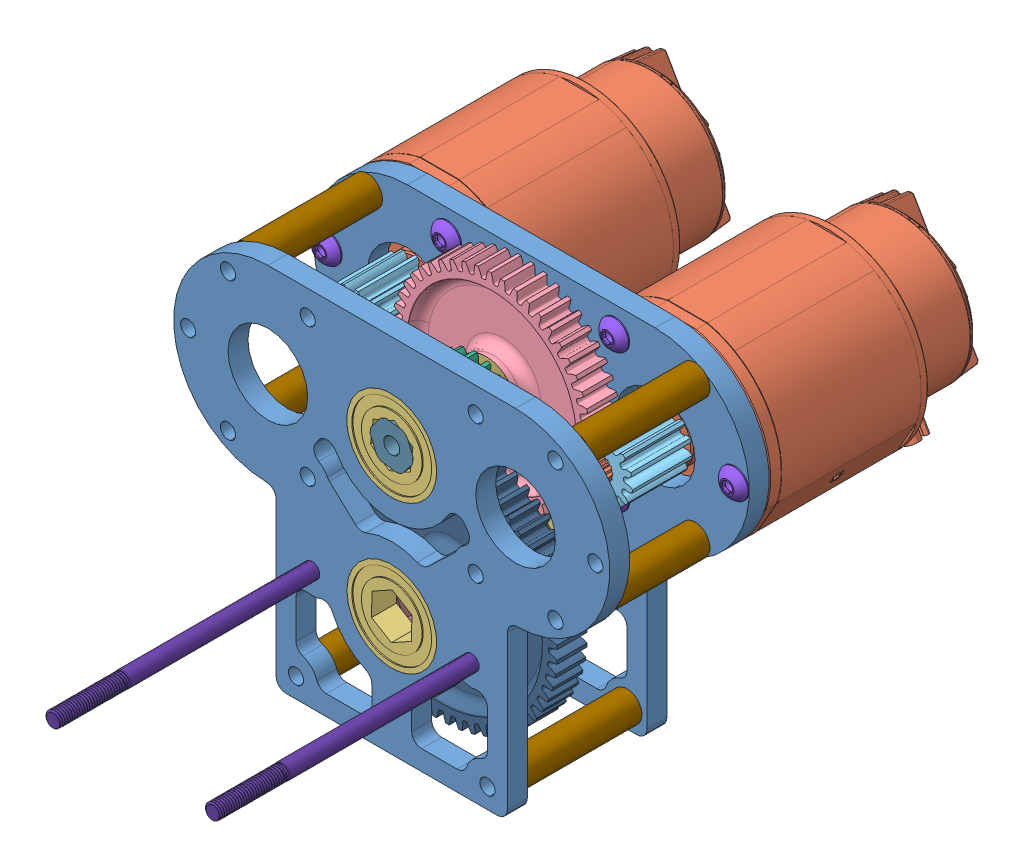
SolidWorks assembly 2 stage elevator gearbox, configuration Default. Lengths in mm.
Overall size (160.87 135.08 215.73).
38 component instances, 17 part files, 79 mates.
Components (placement in the parent):
- 2stage gearbox plate-1: 2stage gearbox plate [Default] at (38.8703 49.9501 110.3319) size (138.89 115.16 6.35)
- Vexpro - Falcon 500 - 217-6515-1: Vexpro - Falcon 500 - 217-6515 [Default] at (74.1311 92.2322 73.3938) x (0.866025 -0.5 0) z (0 0 1) size (60.01 60.01 116.76)
- Vexpro - Falcon 500 - 217-6515-2: Vexpro - Falcon 500 - 217-6515 [Default] at (-4.7613 92.2322 73.3938) x (0.866025 -0.5 0) z (0 0 1) size (60.01 60.01 116.76)
- Vexpro - .5in hex bearing flanged - 217-3875-1: Vexpro - .5in hex bearing flanged - 217-3875 [Default] at (38.8703 97.0163 110.3319) x (0.982389 0.186848 0) z (0.186848 -0.982389 0) size (31.12 7.94 31.12)
- Vexpro - .5in hex bearing flanged - 217-3875-2: Vexpro - .5in hex bearing flanged - 217-3875 [Default] at (38.8703 49.9501 110.3319) x (0.9326 0.360911 0) z (0.360911 -0.9326 0) size (31.12 7.94 31.12)
- 48t pocketed gear-1: 48t pocketed gear [Default] at (38.8703 97.0163 124.594) x (0.984542 -0.175146 0) z (0 0 1) size (63.43 63.43 12.65)
- 14t pinion-1: 14t pinion [Default] at (78.3161 97.0172 124.4944) x (0.865876 0.500258 0) z (0 0 1) size (20.01 20.32 19.05)
- 14t pinion-2: 14t pinion [Default] at (-0.5766 97.0171 124.4944) x (0.709301 0.704906 0) z (0 0 1) size (20.01 20.32 19.05)
- Vexpro - 18t 20DP .5 Hex Gear - 217-5460-1: Vexpro - 18t 20DP .5 Hex Gear - 217-5460 [Default] at (38.8703 97.0163 140.5444) x (0.941397 0.3373 0) z (0 0 1) size (25.18 25.4 12.6)
- Vexpro - .5in acetal hex spacer - 217 - 3261-1: Vexpro - .5in acetal hex spacer - 217 - 3261 [Default] at (38.8703 49.9501 124.6194) x (-0.39458 0.918862 0) z (0 0 1) size (19.5 19.5 12.7)
- 2stage gearbox plate-2: 2stage gearbox plate [outside] at (38.8703 49.9501 154.7819) size (138.89 115.16 6.35)
- Vexpro - .5in hex bearing flanged - 217-3875-4: Vexpro - .5in hex bearing flanged - 217-3875 [Default] at (38.8703 49.9501 161.1319) x (-0.017353 -0.999849 0) z (0.999849 -0.017353 0) size (31.12 7.94 31.12)
- Vexpro - .5in hex bearing flanged - 217-3875-5: Vexpro - .5in hex bearing flanged - 217-3875 [Default] at (38.8703 97.0163 161.1319) x (-0.113044 -0.99359 0) z (0.99359 -0.113044 0) size (31.12 7.94 31.12)
- McMaster - 10-32 .3125in button head screw - 97763A706-2: McMaster - 10-32 .3125in button head screw - 97763A706 [97763A706] at (12.1241 119.0134 113.9959) size (9.17 9.17 10.95)
- McMaster - 10-32 .3125in button head screw - 97763A706-3: McMaster - 10-32 .3125in button head screw - 97763A706 [97763A706] at (12.1241 75.0193 113.9959) size (9.17 9.17 10.95)
- McMaster - 10-32 .3125in button head screw - 97763A706-4: McMaster - 10-32 .3125in button head screw - 97763A706 [97763A706] at (-25.9759 97.0163 113.9959) size (9.17 9.17 10.95)
- McMaster - 10-32 .3125in button head screw - 97763A706-5: McMaster - 10-32 .3125in button head screw - 97763A706 [97763A706] at (-13.2759 75.0193 113.9959) size (9.17 9.17 10.95)
- McMaster - 10-32 .3125in button head screw - 97763A706-9: McMaster - 10-32 .3125in button head screw - 97763A706 [97763A706] at (103.7165 97.0163 113.9959) size (9.17 9.17 10.95)
- McMaster - 10-32 .3125in button head screw - 97763A706-10: McMaster - 10-32 .3125in button head screw - 97763A706 [97763A706] at (65.6165 75.0193 113.9959) size (9.17 9.17 10.95)
- McMaster - 10-32 .3125in button head screw - 97763A706-12: McMaster - 10-32 .3125in button head screw - 97763A706 [97763A706] at (65.6165 119.0134 113.9959) size (9.17 9.17 10.95)
- McMaster - 10-32 .3125in button head screw - 97763A706-13: McMaster - 10-32 .3125in button head screw - 97763A706 [97763A706] at (8.3903 18.2001 113.018) x (-0.932553 0.361034 0) z (0 0 -1) size (9.17 9.17 10.95)
- McMaster - 10-32 .3125in button head screw - 97763A706-15: McMaster - 10-32 .3125in button head screw - 97763A706 [97763A706] at (69.3503 18.2001 113.018) x (-0.932553 0.361034 0) z (0 0 -1) size (9.17 9.17 10.95)
- 1.5in gearbox spacer-1: 1.5in gearbox spacer [Default] at (69.3503 18.2001 154.7819) x (-0.965755 0.259455 0) z (-0.259455 -0.965755 0) size (9.53 38.1 9.53)
- 1.5in gearbox spacer-2: 1.5in gearbox spacer [Default] at (8.3903 18.2001 154.7819) x (-0.965755 0.259455 0) z (-0.259455 -0.965755 0) size (9.53 38.1 9.53)
- 1.5in gearbox spacer-3: 1.5in gearbox spacer [Default] at (91.0165 119.0134 154.7819) x (-0.883824 -0.46782 0) z (0.46782 -0.883824 0) size (9.53 38.1 9.53)
- 1.5in gearbox spacer-4: 1.5in gearbox spacer [Default] at (-13.2759 119.0134 154.7819) x (-0.965755 0.259455 0) z (-0.259455 -0.965755 0) size (9.53 38.1 9.53)
- 1.5in gearbox spacer-5: 1.5in gearbox spacer [Default] at (-13.2759 75.0193 154.7819) x (-0.965755 0.259455 0) z (-0.259455 -0.965755 0) size (9.53 38.1 9.53)
- 56t pocketed gear-1: 56t pocketed gear [Default] at (38.8703 49.9501 140.4444) x (0.941864 -0.335993 0) z (0 0 1) size (73.6 73.6 12.6)
- Clamping Shaft Collar - 1_2 Hex ID (217-2737)-1: Clamping Shaft Collar - 1_2 Hex ID (217-2737) [Default] at (38.8703 97.0163 150.0194) x (0.340948 -0.940082 0) z (0 0 1) size (25.39 25.4 6.35)
- Vexpro - .125 acetal hex spacer - 217-2758-1: Vexpro - .125 acetal hex spacer - 217-2758 [Default] at (38.8703 49.9501 132.5569) x (0.658563 0.752525 0) z (0 0 1) size (19.05 19.05 3.17)
- Vexpro - .125 acetal hex spacer - 217-2758-2: Vexpro - .125 acetal hex spacer - 217-2758 [Default] at (38.8703 97.0163 132.6569) x (0.658563 0.752525 0) z (0 0 1) size (19.05 19.05 3.17)
- Vexpro - .25in acetal hex spacer - 217-3259-1: Vexpro - .25in acetal hex spacer - 217-3259 [Default] at (38.8703 49.9501 150.0194) size (19.5 19.5 6.35)
- 2in hex axle-1: 2in hex axle [Default] at (64.1668 94.7262 213.5194) x (0.995927 -0.090161 0) z (0 0 1) size (14.65 14.61 50.8)
- McMaster - .25 ID washer - 96765A140-1: McMaster - .25 ID washer - 96765A140 [96765A140] at (38.8703 97.0163 110.3319) x (1 0 0) z (0 1 0) size (15.88 1.52 15.88)
- McMaster - .25-20 .5in socket head - 91251A537-1: McMaster - .25-20 .5in socket head - 91251A537 [91251A537] at (38.8703 97.0163 121.5079) size (9.53 9.53 20.44)
- McMaster 10-32 3.tin socket Head 91251A361_Black-Oxide Alloy Steel Socket Head Screw-2: McMaster 10-32 3.tin socket Head 91251A361_Black-Oxide Alloy Steel Socket Head Screw [91251A361] at (13.4703 49.9501 196.8189) x (0.923728 0.383049 0) z (0 0 -1) size (7.94 7.94 94.22)
- McMaster 10-32 3.tin socket Head 91251A361_Black-Oxide Alloy Steel Socket Head Screw-3: McMaster 10-32 3.tin socket Head 91251A361_Black-Oxide Alloy Steel Socket Head Screw [91251A361] at (64.2703 49.9501 196.8189) x (0.923728 0.383049 0) z (0 0 -1) size (7.94 7.94 94.22)
- 1.5in gearbox spacer-6: 1.5in gearbox spacer [Default] at (91.0165 75.0193 154.7819) x (-0.883824 -0.46782 0) z (0.46782 -0.883824 0) size (9.53 38.1 9.53)
Mates (geometry in assembly coordinates):
- Concentric1: concentric aligned: cylinder of Vexpro - Falcon 500 - 217-6515-1 through (78.3165 97.0163 106.3319) axis (0 0 -1) radius 30; cylinder of 2stage gearbox plate-1 through (78.3165 97.0163 116.6819) axis (0 0 -1) radius 29.9974
- Concentric2: concentric aligned: cylinder of Vexpro - Falcon 500 - 217-6515-2 through (-0.5759 97.0163 106.3319) axis (0 0 -1) radius 30; cylinder of 2stage gearbox plate-1 through (-0.5759 97.0163 116.6819) axis (0 0 -1) radius 29.9974
- Coincident1: coincident anti-aligned: plane of 2stage gearbox plate-1 through (38.8703 49.9501 110.3319) normal (0 0 -1); plane of Vexpro - Falcon 500 - 217-6515-2 through (-8.8248 92.2538 110.3319) normal (0 0 1)
- Coincident2: coincident anti-aligned: plane of 2stage gearbox plate-1 through (38.8703 49.9501 110.3319) normal (0 0 -1); plane of Vexpro - Falcon 500 - 217-6515-1 through (70.0676 92.2538 110.3319) normal (0 0 1)
- Coincident3: coincident anti-aligned: plane of 2stage gearbox plate-1 through (38.8703 49.9501 116.6819) normal (0 0 1); plane of Vexpro - .5in hex bearing flanged - 217-3875-1 through (54.1538 99.9232 116.6819) normal (0 0 -1)
- Coincident4: coincident anti-aligned: plane of 2stage gearbox plate-1 through (38.8703 49.9501 116.6819) normal (0 0 1); plane of Vexpro - .5in hex bearing flanged - 217-3875-2 through (53.3792 55.565 116.6819) normal (0 0 -1)
- Concentric6: concentric anti-aligned: circle of Vexpro - .5in hex bearing flanged - 217-3875-1; unknown of 48t pocketed gear-1
- Concentric7: concentric: point of Vexpro - Falcon 500 - 217-6515-1; unknown of 14t pinion-1
- Coincident6: coincident anti-aligned: plane of Vexpro - Falcon 500 - 217-6515-1 through (80.4098 94.8914 114.9694) normal (0 0 1); plane of 14t pinion-1 through (73.2334 105.8145 114.9694) normal (0 0 -1)
- Concentric8: concentric: cylinder of Vexpro - Falcon 500 - 217-6515-2 through (-0.5759 97.0163 145.1319) axis (0 0 1) radius 1.7272; unknown of 14t pinion-2
- Coincident8: coincident anti-aligned: plane of Vexpro - Falcon 500 - 217-6515-2 through (1.5174 94.8914 114.9694) normal (0 0 1); plane of 14t pinion-2 through (-7.7384 104.2236 114.9694) normal (0 0 -1)
- Concentric11: concentric aligned: unknown of 48t pocketed gear-1; unknown of Vexpro - 18t 20DP .5 Hex Gear - 217-5460-1
- Concentric12: concentric anti-aligned: unknown of Vexpro - .5in hex bearing flanged - 217-3875-2; cylinder of Vexpro - .5in acetal hex spacer - 217 - 3261-1 through (38.8703 49.9501 130.9694) axis (0 0 -1) radius 9.75
- Concentric13: concentric aligned: unknown of Vexpro - 18t 20DP .5 Hex Gear - 217-5460-1; cylinder of 2stage gearbox plate-2 through (38.8703 97.0163 161.1319) axis (0 0 -1) radius 14.2875
- Concentric14: concentric anti-aligned: cylinder of Vexpro - Falcon 500 - 217-6515-2 through (-0.5759 97.0163 145.1319) axis (0 0 1) radius 1.7272; cylinder of 2stage gearbox plate-2 through (-0.5759 97.0163 161.1319) axis (0 0 -1) radius 12.7
- Concentric15: concentric aligned: cylinder of 2stage gearbox plate-2 through (38.8703 49.9501 161.1319) axis (0 0 -1) radius 14.2875; cylinder of Vexpro - .5in hex bearing flanged - 217-3875-4 through (38.8703 49.9501 161.1319) axis (0 0 -1) radius 14.2748
- Coincident12: coincident anti-aligned: plane of 2stage gearbox plate-2 through (38.8703 49.9501 154.7819) normal (0 0 -1); plane of Vexpro - .5in hex bearing flanged - 217-3875-4 through (38.6003 34.395 154.7819) normal (0 0 1)
- Concentric16: concentric aligned: cylinder of Vexpro - .5in hex bearing flanged - 217-3875-5 through (38.8703 97.0163 161.1319) axis (0 0 -1) radius 14.2748; cylinder of 2stage gearbox plate-2 through (38.8703 97.0163 161.1319) axis (0 0 -1) radius 14.2875
- Coincident13: coincident anti-aligned: plane of 2stage gearbox plate-2 through (38.8703 49.9501 154.7819) normal (0 0 -1); plane of Vexpro - .5in hex bearing flanged - 217-3875-5 through (37.1116 81.5585 154.7819) normal (0 0 1)
- Concentric17: concentric aligned: unknown of Vexpro - Falcon 500 - 217-6515-2; unknown of McMaster - 10-32 .3125in button head screw - 97763A706-4
- Concentric18: concentric aligned: unknown of Vexpro - Falcon 500 - 217-6515-1; unknown of McMaster - 10-32 .3125in button head screw - 97763A706-12
- Concentric21: concentric aligned: cylinder of 2stage gearbox plate-1 through (12.1241 119.0134 110.3319) axis (0 0 1) radius 2.413; unknown of McMaster - 10-32 .3125in button head screw - 97763A706-2
- Coincident18: coincident anti-aligned: plane of 2stage gearbox plate-1 through (38.8703 49.9501 116.6819) normal (0 0 1); plane of McMaster - 10-32 .3125in button head screw - 97763A706-2 through (12.1241 123.5981 116.6819) normal (0 0 -1)
- Coincident19: coincident anti-aligned: plane of 2stage gearbox plate-1 through (38.8703 49.9501 116.6819) normal (0 0 1); plane of McMaster - 10-32 .3125in button head screw - 97763A706-3 through (12.1241 79.604 116.6819) normal (0 0 -1)
- Concentric22: concentric aligned: cylinder of 2stage gearbox plate-1 through (12.1241 75.0193 110.3319) axis (0 0 1) radius 2.413; unknown of McMaster - 10-32 .3125in button head screw - 97763A706-3
- Concentric23: concentric aligned: cylinder of 2stage gearbox plate-1 through (-25.9759 97.0163 110.3319) axis (0 0 1) radius 2.413; unknown of McMaster - 10-32 .3125in button head screw - 97763A706-4
- Coincident20: coincident anti-aligned: plane of 2stage gearbox plate-1 through (38.8703 49.9501 116.6819) normal (0 0 1); plane of McMaster - 10-32 .3125in button head screw - 97763A706-4 through (-25.9759 101.601 116.6819) normal (0 0 -1)
- Concentric24: concentric aligned: cylinder of 2stage gearbox plate-1 through (-13.2759 75.0193 110.3319) axis (0 0 1) radius 2.413; unknown of McMaster - 10-32 .3125in button head screw - 97763A706-5
- Coincident21: coincident anti-aligned: plane of 2stage gearbox plate-1 through (38.8703 49.9501 116.6819) normal (0 0 1); plane of McMaster - 10-32 .3125in button head screw - 97763A706-5 through (-13.2759 79.604 116.6819) normal (0 0 -1)
- Coincident23: coincident anti-aligned: plane of 2stage gearbox plate-1 through (38.8703 49.9501 116.6819) normal (0 0 1); plane of McMaster - 10-32 .3125in button head screw - 97763A706-12 through (65.6165 123.5981 116.6819) normal (0 0 -1)
- Concentric27: concentric aligned: cylinder of 2stage gearbox plate-1 through (65.6165 119.0134 110.3319) axis (0 0 1) radius 2.413; unknown of McMaster - 10-32 .3125in button head screw - 97763A706-12
- Coincident25: coincident anti-aligned: plane of 2stage gearbox plate-1 through (38.8703 49.9501 116.6819) normal (0 0 1); plane of McMaster - 10-32 .3125in button head screw - 97763A706-9 through (103.7165 101.601 116.6819) normal (0 0 -1)
- Concentric29: concentric aligned: cylinder of 2stage gearbox plate-1 through (103.7165 97.0163 110.3319) axis (0 0 1) radius 2.413; unknown of McMaster - 10-32 .3125in button head screw - 97763A706-9
- Concentric30: concentric aligned: unknown of McMaster - 10-32 .3125in button head screw - 97763A706-10; cylinder of 2stage gearbox plate-1 through (65.6165 75.0193 110.3319) axis (0 0 1) radius 2.413
- Coincident26: coincident anti-aligned: plane of 2stage gearbox plate-1 through (38.8703 49.9501 116.6819) normal (0 0 1); plane of McMaster - 10-32 .3125in button head screw - 97763A706-10 through (65.6165 79.604 116.6819) normal (0 0 -1)
- Coincident28: coincident anti-aligned: plane of 2stage gearbox plate-1 through (38.8703 49.9501 110.3319) normal (0 0 -1); plane of McMaster - 10-32 .3125in button head screw - 97763A706-13 through (10.0455 22.4756 110.3319) normal (0 0 1)
- Concentric32: concentric aligned: unknown of McMaster - 10-32 .3125in button head screw - 97763A706-13; unknown of 2stage gearbox plate-1
- Coincident29: coincident anti-aligned: plane of 2stage gearbox plate-1 through (38.8703 49.9501 110.3319) normal (0 0 -1); plane of McMaster - 10-32 .3125in button head screw - 97763A706-15 through (71.0055 22.4756 110.3319) normal (0 0 1)
- Concentric33: concentric aligned: unknown of McMaster - 10-32 .3125in button head screw - 97763A706-15; cylinder of 2stage gearbox plate-1 through (69.3503 18.2001 116.6819) axis (0 0 -1) radius 2.413
- Concentric40: concentric anti-aligned: cylinder of 1.5in gearbox spacer-1 through (69.3503 18.2001 116.6819) axis (0 0 1) radius 4.7625; cylinder of 2stage gearbox plate-2 through (69.3503 18.2001 161.1319) axis (0 0 -1) radius 2.413
- Coincident37: coincident anti-aligned: plane of 2stage gearbox plate-2 through (38.8703 49.9501 154.7819) normal (0 0 -1); plane of 1.5in gearbox spacer-1 through (69.3503 18.2001 154.7819) normal (0 0 1)
- Coincident38: coincident anti-aligned: plane of 2stage gearbox plate-1 through (38.8703 49.9501 116.6819) normal (0 0 1); plane of 1.5in gearbox spacer-1 through (69.3503 18.2001 116.6819) normal (0 0 -1)
- Concentric41: concentric anti-aligned: cylinder of 1.5in gearbox spacer-2 through (8.3903 18.2001 116.6819) axis (0 0 1) radius 4.7625; unknown of 2stage gearbox plate-2
- Coincident39: coincident anti-aligned: plane of 2stage gearbox plate-2 through (38.8703 49.9501 154.7819) normal (0 0 -1); plane of 1.5in gearbox spacer-2 through (8.3903 18.2001 154.7819) normal (0 0 1)
- Concentric42: concentric aligned: cylinder of 1.5in gearbox spacer-3 through (91.0165 119.0134 116.6819) axis (0 0 1) radius 4.7625; unknown of 2stage gearbox plate-1
- Coincident40: coincident anti-aligned: plane of 2stage gearbox plate-2 through (38.8703 49.9501 154.7819) normal (0 0 -1); plane of 1.5in gearbox spacer-3 through (91.0165 119.0134 154.7819) normal (0 0 1)
- Concentric43: concentric aligned: cylinder of 1.5in gearbox spacer-4 through (-13.2759 119.0134 116.6819) axis (0 0 1) radius 4.7625; cylinder of 2stage gearbox plate-1 through (-13.2759 119.0134 110.3319) axis (0 0 1) radius 2.413
- Coincident41: coincident anti-aligned: plane of 2stage gearbox plate-1 through (38.8703 49.9501 116.6819) normal (0 0 1); plane of 1.5in gearbox spacer-4 through (-13.2759 119.0134 116.6819) normal (0 0 -1)
- Coincident42: coincident anti-aligned: plane of 2stage gearbox plate-2 through (38.8703 49.9501 154.7819) normal (0 0 -1); plane of 1.5in gearbox spacer-5 through (-13.2759 75.0193 154.7819) normal (0 0 1)
- Concentric45: concentric aligned: cylinder of 1.5in gearbox spacer-5 through (-13.2759 75.0193 116.6819) axis (0 0 1) radius 4.7625; unknown of 2stage gearbox plate-2
- Coincident46: coincident anti-aligned: plane of Vexpro - .5in hex bearing flanged - 217-3875-2 through (44.7923 52.2419 118.2694) normal (0 0 1); plane of Vexpro - .5in acetal hex spacer - 217 - 3261-1 through (38.8703 49.9501 118.2694) normal (0 0 -1)
- Concentric48: concentric anti-aligned: unknown of Vexpro - .5in acetal hex spacer - 217 - 3261-1; unknown of 56t pocketed gear-1
- Concentric50: concentric aligned: cylinder of Vexpro - .5in hex bearing flanged - 217-3875-5 through (38.8703 97.0163 161.1319) axis (0 0 -1) radius 15.5575; cylinder of Clamping Shaft Collar - 1_2 Hex ID (217-2737)-1 through (38.8703 97.0163 153.1944) axis (0 0 -1) radius 12.7
- Coincident54: coincident anti-aligned: plane of Vexpro - .5in hex bearing flanged - 217-3875-5 through (38.1525 90.707 153.1944) normal (0 0 -1); plane of Clamping Shaft Collar - 1_2 Hex ID (217-2737)-1 through (38.8703 97.0163 153.1944) normal (0 0 1)
- Coincident56: coincident anti-aligned: plane of Vexpro - 18t 20DP .5 Hex Gear - 217-5460-1 through (38.8703 97.0163 146.8444) normal (0 0 1); plane of Clamping Shaft Collar - 1_2 Hex ID (217-2737)-1 through (38.8703 97.0163 146.8444) normal (0 0 -1)
- Coincident58: coincident aligned: plane of Vexpro - .5in hex bearing flanged - 217-3875-1 through (45.1085 98.2028 118.2694) normal (0 0 1); circle of 48t pocketed gear-1
- Concentric52: concentric aligned: cylinder of Vexpro - .5in acetal hex spacer - 217 - 3261-1 through (38.8703 49.9501 130.9694) axis (0 0 -1) radius 9.75; cylinder of Vexpro - .125 acetal hex spacer - 217-2758-1 through (38.8703 49.9501 134.1444) axis (0 0 -1) radius 9.525
- Coincident59: coincident aligned: circle of 56t pocketed gear-1; plane of Vexpro - .125 acetal hex spacer - 217-2758-1 through (38.8703 49.9501 134.1444) normal (0 0 1)
- Coincident60: coincident aligned: plane of Vexpro - .5in acetal hex spacer - 217 - 3261-1 through (38.8703 49.9501 130.9694) normal (0 0 1); circle of Vexpro - .125 acetal hex spacer - 217-2758-1
- Concentric53: concentric aligned: cylinder of 48t pocketed gear-1 through (38.8703 97.0163 130.9186) axis (0 0 -1) radius 8.89; cylinder of Vexpro - .125 acetal hex spacer - 217-2758-2 through (38.8703 97.0163 134.2444) axis (0 0 -1) radius 9.525
- Coincident61: coincident anti-aligned: circle of Vexpro - 18t 20DP .5 Hex Gear - 217-5460-1; plane of Vexpro - .125 acetal hex spacer - 217-2758-2 through (38.8703 97.0163 134.2444) normal (0 0 1)
- Concentric54: concentric aligned: cylinder of 56t pocketed gear-1 through (38.8703 49.9501 146.7444) axis (0 0 -1) radius 8.89; cylinder of Vexpro - .25in acetal hex spacer - 217-3259-1 through (38.8703 49.9501 153.1944) axis (0 0 -1) radius 9.75
- Coincident62: coincident anti-aligned: plane of Vexpro - .5in hex bearing flanged - 217-3875-4 through (38.7601 43.6011 153.1944) normal (0 0 -1); circle of Vexpro - .25in acetal hex spacer - 217-3259-1
- Concentric55: concentric aligned: circle of Vexpro - .5in hex bearing flanged - 217-3875-5; cylinder of 2in hex axle-1 through (38.8703 97.0163 110.3319) axis (0 0 -1) radius 2.5527
- Coincident63: coincident aligned: plane of Vexpro - .5in hex bearing flanged - 217-3875-5 through (37.7792 87.4262 161.1319) normal (0 0 1); plane of 2in hex axle-1 through (38.8703 97.0163 161.1319) normal (0 0 1)
- Coincident66: coincident anti-aligned: plane of 2in hex axle-1 through (38.8703 97.0163 110.3319) normal (0 0 -1); plane of McMaster - .25 ID washer - 96765A140-1 through (38.8703 97.0163 110.3319) normal (0 0 1)
- Concentric57: concentric aligned: cylinder of 2in hex axle-1 through (38.8703 97.0163 110.3319) axis (0 0 -1) radius 2.5527; cylinder of McMaster - .25 ID washer - 96765A140-1 through (38.8703 97.0163 110.3319) axis (0 0 -1) radius 3.5687
- Concentric58: concentric anti-aligned: cylinder of McMaster - .25 ID washer - 96765A140-1 through (38.8703 97.0163 110.3319) axis (0 0 -1) radius 3.5687; cylinder of McMaster - .25-20 .5in socket head - 91251A537-1 through (38.8703 97.0163 102.4579) axis (0 0 1) radius 4.7625
- Coincident67: coincident anti-aligned: plane of McMaster - .25 ID washer - 96765A140-1 through (38.8703 97.0163 108.8079) normal (0 0 -1); circle of McMaster - .25-20 .5in socket head - 91251A537-1
- Concentric591: concentric aligned: cylinder of McMaster 10-32 3.tin socket Head 91251A361_Black-Oxide Alloy Steel Socket Head Screw-2 through (13.4703 49.9501 147.8132) axis (0 0 1) radius 2.4638; cylinder of 2stage gearbox plate-2 through (13.4703 49.9501 154.7819) axis (0 0 1) radius 2.413
- Coincident681: coincident anti-aligned: plane of 2stage gearbox plate-2 through (38.8703 49.9501 154.7819) normal (0 0 -1); plane of McMaster 10-32 3.tin socket Head 91251A361_Black-Oxide Alloy Steel Socket Head Screw-2 through (14.3946 47.7212 154.7819) normal (0 0 1)
- Concentric601: concentric aligned: cylinder of 2stage gearbox plate-2 through (64.2703 49.9501 154.7819) axis (0 0 1) radius 2.413; cylinder of McMaster 10-32 3.tin socket Head 91251A361_Black-Oxide Alloy Steel Socket Head Screw-3 through (64.2703 49.9501 147.8132) axis (0 0 1) radius 2.4638
- Coincident691: coincident anti-aligned: plane of 2stage gearbox plate-2 through (38.8703 49.9501 154.7819) normal (0 0 -1); plane of McMaster 10-32 3.tin socket Head 91251A361_Black-Oxide Alloy Steel Socket Head Screw-3 through (65.1946 47.7212 154.7819) normal (0 0 1)
- Concentric602: concentric aligned: circle of 2stage gearbox plate-2; circle of 56t pocketed gear-1
- Concentric603: concentric aligned: cylinder of 2stage gearbox plate-1 through (38.8703 97.0163 116.6819) axis (0 0 -1) radius 14.2875; cylinder of 2stage gearbox plate-2 through (38.8703 97.0163 161.1319) axis (0 0 -1) radius 14.2875
- Concentric604: concentric aligned: cylinder of 2stage gearbox plate-2 through (38.8703 97.0163 161.1319) axis (0 0 -1) radius 14.2875; cylinder of Vexpro - .5in hex bearing flanged - 217-3875-5 through (38.8703 97.0163 161.1319) axis (0 0 -1) radius 14.2748
- Coincident692: coincident anti-aligned: cylinder of 2stage gearbox plate-1 through (38.8703 49.9501 116.6819) axis (0 0 -1) radius 14.2875; circle of 2stage gearbox plate-2
- Concentric6051: concentric aligned: cylinder of 2stage gearbox plate-1 through (91.0165 75.0193 110.3319) axis (0 0 1) radius 2.413; cylinder of 1.5in gearbox spacer-6 through (91.0165 75.0193 116.6819) axis (0 0 1) radius 4.7625
- Coincident693: coincident anti-aligned: plane of 2stage gearbox plate-2 through (38.8703 49.9501 154.7819) normal (0 0 -1); plane of 1.5in gearbox spacer-6 through (91.0165 75.0193 154.7819) normal (0 0 1)
